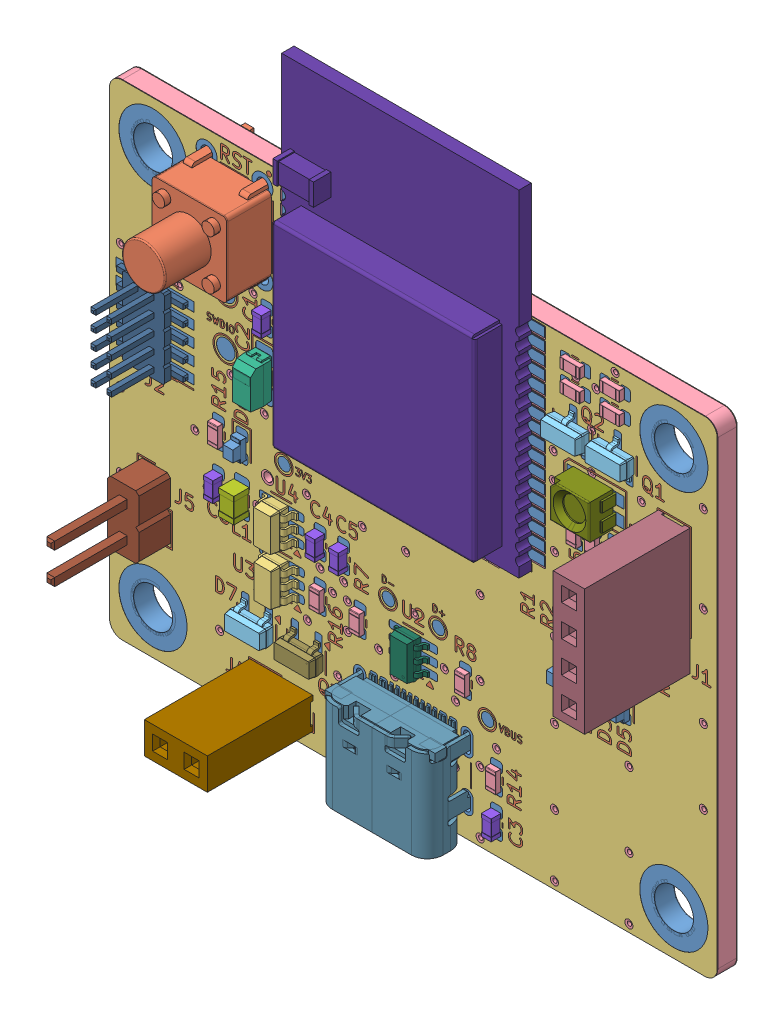
SolidWorks assembly UWBkit_minimal, configuration Default. Lengths in mm.
Overall size (49.01 48.45 15.4).
49 component instances, 22 part files, 0 mates.
Components (placement in the parent):
- UWBkit_minimal.step-1: UWBkit_minimal.step [Default] at origin size (49.01 48.45 15.4)
  - LED_0603_1608Metric.step-1: LED_0603_1608Metric.step [Default] at (168.7 -85.925 1.595) x (0 -1 0) z (0 0 1) size (1.6 0.8 1.1)
  - SW_PUSH_6mm_H7.3mm.step-1: SW_PUSH_6mm_H7.3mm.step [Default] at (139.45 -64.15 1.595) x (0 -1 0) z (0 0 1) size (7.17 6 10.8)
  - SOT-23-5.step-1: SOT-23-5.step [Default] at (141 -86.775 1.595) x (-1 0 0) z (0 0 1) size (2.8 2.9 1.55)
  - R_0603_1608Metric.step-1: R_0603_1608Metric.step [Default] at (165.5 -82.3 1.595) x (0 1 0) z (0 0 1) size (1.6 0.8 0.45)
  - R_0603_1608Metric.step-2: R_0603_1608Metric.step [Default] at (135.9 -83.2 1.595) x (0 -1 0) z (0 0 1) size (1.6 0.8 0.45)
  - R_0603_1608Metric.step-3: R_0603_1608Metric.step [Default] at (163.9 -82.3 1.595) x (0 1 0) z (0 0 1) size (1.6 0.8 0.45)
  - SOT-23.step-1: SOT-23.step [Default] at (168.1 -68.7 1.595) x (0 1 0) z (0 0 1) size (2.5 3 1.2)
  - CP_EIA-3216-18_Kemet-A.step-1: CP_EIA-3216-18_Kemet-A.step [Default] at (139.6 -77.2775 1.595) x (0 -1 0) z (0 0 1) size (3.2 1.6 1.8)
  - L_0805_2012Metric.step-1: L_0805_2012Metric.step [Default] at (137.8 -86.8 1.595) x (0 1 0) z (0 0 1) size (2 1.25 1.25)
  - C_0603_1608Metric.step-1: C_0603_1608Metric.step [Default] at (139.8 -73.325 1.595) x (0 1 0) z (0 0 1) size (1.6 0.8 0.8)
  - PinSocket_1x02_P2.54mm_Vertical.step-1: PinSocket_1x02_P2.54mm_Vertical.step [Default] at (142.275 -99 1.595) x (0 -1 0) z (0 0 1) size (2.54 5.08 11.6)
  - R_0603_1608Metric.step-4: R_0603_1608Metric.step [Default] at (167.9 -65.8 1.595) x (-1 0 0) z (0 0 1) size (1.6 0.8 0.45)
  - C_0603_1608Metric.step-2: C_0603_1608Metric.step [Default] at (146 -86.8 1.595) x (0 -1 0) z (0 0 1) size (1.6 0.8 0.8)
  - PinHeader_2x05_P1.27mm_Vertical_SMD.step-1: PinHeader_2x05_P1.27mm_Vertical_SMD.step [Default] at (130.8 -78 1.595) x (-1 0 0) z (0 0 1) size (5.57 6.35 4.4)
  - R_0603_1608Metric.step-5: R_0603_1608Metric.step [Default] at (167.8 -75.7 1.595) x (0 1 0) z (0 0 1) size (1.6 0.8 0.45)
  - SOT-23.step-2: SOT-23.step [Default] at (164.5 -68.7 1.595) x (0 1 0) z (0 0 1) size (2.5 3 1.2)
  - PinHeader_1x02_P2.54mm_Vertical.step-1: PinHeader_1x02_P2.54mm_Vertical.step [Default] at (130.8 -89.325 1.595) size (2.54 5.08 11.54)
  - R_0603_1608Metric.step-6: R_0603_1608Metric.step [Default] at (164.8 -75.7 1.595) x (0 1 0) z (0 0 1) size (1.6 0.8 0.45)
  - SOT-23-3.step-1: SOT-23-3.step [Default] at (143.025 -95 1.595) x (0 -1 0) z (0 0 1) size (2.5 3 1.2)
  - PinSocket_1x04_P2.54mm_Vertical.step-1: PinSocket_1x04_P2.54mm_Vertical.step [Default] at (172.7 -79.745 1.595) x (-1 0 0) z (0 0 1) size (2.54 10.16 11.6)
  - R_0603_1608Metric.step-7: R_0603_1608Metric.step [Default] at (164.7 -65.8 1.595) size (1.6 0.8 0.45)
  - LED_0603_1608Metric.step-2: LED_0603_1608Metric.step [Default] at (163.9 -85.925 1.595) x (0 -1 0) z (0 0 1) size (1.6 0.8 1.1)
  - SOT-23.step-3: SOT-23.step [Default] at (139.025 -95 1.595) x (0 -1 0) z (0 0 1) size (2.5 3 1.2)
  - R_0603_1608Metric.step-8: R_0603_1608Metric.step [Default] at (166.3 -75.7 1.595) x (0 1 0) z (0 0 1) size (1.6 0.8 0.45)
  - SOT-23-5.step-2: SOT-23-5.step [Default] at (141.025 -90.6 1.595) x (-1 0 0) z (0 0 1) size (2.8 2.9 1.55)
  - R_0603_1608Metric.step-9: R_0603_1608Metric.step [Default] at (167.9 -64.1 1.595) size (1.6 0.8 0.45)
  - USB_C_Receptacle_GCT_USB4105-xx-A_16P_TopMnt_Horizontal.step-1: USB_C_Receptacle_GCT_USB4105-xx-A_16P_TopMnt_Horizontal.step [Default] at (151.625 -97.94 1.595) size (8.94 7.78 4.26)
  - R_0603_1608Metric.step-10: R_0603_1608Metric.step [Default] at (155.825 -90.6 1.595) x (0 1 0) z (0 0 1) size (1.6 0.8 0.45)
  - C_0603_1608Metric.step-3: C_0603_1608Metric.step [Default] at (144.1 -86.8 1.595) x (0 -1 0) z (0 0 1) size (1.6 0.8 0.8)
  - R_0603_1608Metric.step-11: R_0603_1608Metric.step [Default] at (167.11 -82.3 1.595) x (0 1 0) z (0 0 1) size (1.6 0.8 0.45)
  - C_0603_1608Metric.step-4: C_0603_1608Metric.step [Default] at (135.9 -86.8 1.595) x (0 -1 0) z (0 0 1) size (1.6 0.8 0.8)
  - LED_0603_1608Metric.step-3: LED_0603_1608Metric.step [Default] at (165.5 -85.925 1.595) x (0 -1 0) z (0 0 1) size (1.6 0.8 1.1)
  - LED_0603_1608Metric.step-4: LED_0603_1608Metric.step [Default] at (167.11 -85.925 1.595) x (0 -1 0) z (0 0 1) size (1.6 0.8 1.1)
  - SC-74-6_1.55x2.9mm_P0.95mm.step-1: SC-74-6_1.55x2.9mm_P0.95mm.step [Default] at (151.625 -90.6 1.595) x (-1 0 0) z (0 0 1) size (2.7 2.9 1.18)
  - R_0603_1608Metric.step-12: R_0603_1608Metric.step [Default] at (144.1 -90.6 1.595) x (0 1 0) z (0 0 1) size (1.6 0.8 0.45)
  - LED_0603_1608Metric.step-5: LED_0603_1608Metric.step [Default] at (137.8 -83.2 1.595) x (0 -1 0) z (0 0 1) size (1.6 0.8 1.1)
  - C_0603_1608Metric.step-5: C_0603_1608Metric.step [Default] at (158.325 -99.2 1.595) x (0 -1 0) z (0 0 1) size (1.6 0.8 0.8)
  - R_0603_1608Metric.step-13: R_0603_1608Metric.step [Default] at (164.7 -64.1 1.595) size (1.6 0.8 0.45)
  - R_0603_1608Metric.step-14: R_0603_1608Metric.step [Default] at (158.325 -96.1 1.595) x (0 1 0) z (0 0 1) size (1.6 0.8 0.45)
  - LED_RGB_Wuerth-PLCC4_3.2x2.8mm_150141M173100.step-1: LED_RGB_Wuerth-PLCC4_3.2x2.8mm_150141M173100.step [Default] at (166.3 -72.5 1.595) size (3.5 2.8 2.05)
  - DWM3001C.step-1: DWM3001C.step [Default] at (151.6 -66.71 2.595) size (19.13 27.1 3.2)
  - R_0603_1608Metric.step-15: R_0603_1608Metric.step [Default] at (168.7 -82.3 1.595) x (0 1 0) z (0 0 1) size (1.6 0.8 0.45)
  - R_0603_1608Metric.step-16: R_0603_1608Metric.step [Default] at (147.325 -90.6 1.595) x (0 1 0) z (0 0 1) size (1.6 0.8 0.45)
  - BatteryHolder_Keystone_1058_1x2032.step-1: BatteryHolder_Keystone_1058_1x2032.step [Default] at (151.625 -82.7 -0.085) x (1 0 0) z (0 0 -1) size (31.86 16 5.08)
  - UWBkit_minimal_pad.step-1: UWBkit_minimal_pad.step [Default] at origin size (47.72 38.11 1.59)
  - UWBkit_minimal_silkscreen.step-1: UWBkit_minimal_silkscreen.step [Default] at origin size (46.73 38.02 1.67)
  - UWBkit_minimal_soldermask.step-1: UWBkit_minimal_soldermask.step [Default] at origin size (49.01 39.11 1.62)
  - UWBkit_minimal_PCB.step-1: UWBkit_minimal_PCB.step [Default] at origin size (49 39.1 1.51)
